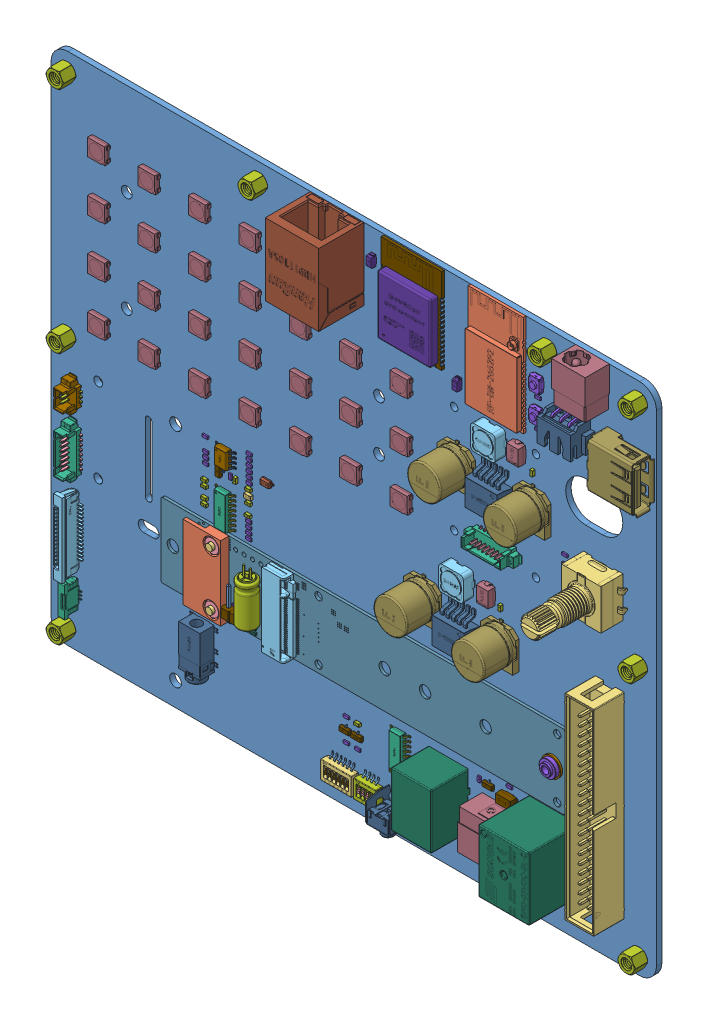
SolidWorks assembly HOUZZkitF1_Tester, configuration 默认. Lengths in mm. (continued)
Components (placement in the parent): (continued)
- HOUZZkitF1_Tester.step-1: HOUZZkitF1_Tester.step [默认] at origin size (180.06 153.05 26.45) (continued)
  - H4.step-1: H4.step [默认] at origin size (25.31 29.5 2.85) (continued)
    - tfcard_test_wire_female.step-1: tfcard_test_wire_female.step [默认] at (-76 20 -1.6) x (0 -1 0) z (0 0 -1) size (29.5 25.31 2.85) (continued)
      - MICRO SD CARD SOCKET.step-1: MICRO SD CARD SOCKET.step [默认] at (119.8236 -42.8675 -195.6897) size (16 17.9 2.44) (continued)
        - MICRO SD CARD SOCKET.step.step-1: MICRO SD CARD SOCKET.step.step [默认] at origin size (16 17.9 2.44) (continued)
          - MOV_SD-13.step.step-1: MOV_SD-13.step.step [默认] at origin size (1.3 1.09 0.1)
          - MOV_SD-14.step.step-1: MOV_SD-14.step.step [默认] at origin size (0.97 1.25 0.1)
          - MOV_SD-15.step.step-1: MOV_SD-15.step.step [默认] at origin size (0.18 0.18 0.1)
      - tfcard_test_wire_female-41.step-1: tfcard_test_wire_female-41.step [默认] at origin size (29.5 22.5 1)
  - LED1.step-1: LED1.step [默认] at origin size (5.4 5 1.7)
    - User Library-WS2812B.step-1: User Library-WS2812B.step [默认] at (-74.9999 93 0.18) x (1 0 0) z (0 -1 0) size (5.4 1.7 5)
  - H3.step-1: H3.step [默认] at origin size (120.05 22.08 8.14)
    - R44SF_bottom.step-1: R44SF_bottom.step [默认] at (-209.2275 115.0408 0.8) x (0 -1 0) z (0 0 1) size (22.08 120.05 8.14)
      - R44SF ..22.step.step-1: R44SF ..22.step.step [默认] at origin size (22.08 120.05 8.14)
        - Board.step.step-1: Board.step.step [默认] at origin size (22.05 120.05 0.8)
          - Open CASCADE STEP translator 6.8 12.1.1.step.step-1: Open CASCADE STEP translator 6.8 12.1.1.step.step [默认] at (0 0 -0.8) size (22.05 120.05 0.8)
        - R3.step.step-1: R3.step.step [默认] at origin size (1.6 0.8 0.45)
          - ________R0603.step.step-1: ________R0603.step.step [默认] at (119.5501 177.9636 0) x (1 0 0) z (0 0 1) size (1.6 0.8 0.45)
            - ________R0603-0.step.step-1: ________R0603-0.step.step [默认] at origin size (1.6 0.8 0.45)
        - D1.step.step-1: D1.step.step [默认] at origin size (0.8 1.6 1.1)
          - LED_AP1608.step.step-1: LED_AP1608.step.step [默认] at (120.3536 180.4092 0) x (0 1 0) z (1 0 0) size (1.6 1.1 0.8)
        - R2.step.step-1: R2.step.step [默认] at origin size (0.8 1.6 0.45)
          - ________R0603.step.step-1: ________R0603.step.step [默认] at (121.7526 180.421 0) x (0 -1 0) z (0 0 1) size (1.6 0.8 0.45)
            - ________R0603-0.step.step-1: ________R0603-0.step.step [默认] at origin size (1.6 0.8 0.45)
        - R1.step.step-1: R1.step.step [默认] at origin size (0.8 1.6 0.45)
          - ________R0603.step.step-1: ________R0603.step.step [默认] at (123.1496 180.421 0) x (0 -1 0) z (0 0 1) size (1.6 0.8 0.45)
            - ________R0603-0.step.step-1: ________R0603-0.step.step [默认] at origin size (1.6 0.8 0.45)
        - Q1.step.step-1: Q1.step.step [默认] at origin size (3 2.55 1)
          - SOT-23.step.step-1: SOT-23.step.step [默认] at (113.165 176.0289 0) x (-1 0 0) z (0 0 1) size (3 2.55 1)
        - Free-Models.step.step-1: Free-Models.step.step [默认] at origin size (22.05 110.48 8.14)
          - bg075-02x-1-0600-0300-0150-x-x_revd.step.step-1: bg075-02x-1-0600-0300-0150-x-x_revd.step.step [默认] at (120.1725 176.0952 0.5) x (0 -1 0) z (0 0 -1) size (5.08 10.36 5.5)
            - BG075-Insulator.step.step-1: BG075-Insulator.step.step [默认] at (0.3712 -0.9743 -0.1079) size (2.54 2.54 2.5)
            - BG075-Insulator.step.step-2: BG075-Insulator.step.step [默认] at (-2.1688 -0.9743 -0.1079) size (2.54 2.54 2.5)
            - BG075-1-0600-0300-0150-pin.step.step-1: BG075-1-0600-0300-0150-pin.step.step [默认] at (1.0892 -2.7943 -1.0379) size (0.64 10.36 4.57)
            - BG075-1-0600-0300-0150-pin.step.step-2: BG075-1-0600-0300-0150-pin.step.step [默认] at (-1.4508 -2.7943 -1.0379) size (0.64 10.36 4.57)
          - RP44S-PAD.step.step-1: RP44S-PAD.step.step [默认] at (102.0666 172.9244 2.5) x (-1 0 0) z (0 -1 0) size (22 2.5 11.2)
          - G0033_RGB9411503.step.step-1: G0033_RGB9411503.step.step [默认] at (121.2666 170.1244 -1.8) x (-1 0 0) z (0 1 0) size (3.3 5 3.3)
          - Hexagon_nut_ISO_4032_(DIN_934)_-_M2_RGB9411503.step.step-1: Hexagon_nut_ISO_4032_(DIN_934)_-_M2_RGB9411503.step.step [默认] at (121.2666 170.1244 1.5) x (-1 0 0) z (0 1 0) size (4.62 1.6 4.62)
          - Hexagon_nut_ISO_4032_(DIN_934)_-_M2_RGB9411503.step.step-2: Hexagon_nut_ISO_4032_(DIN_934)_-_M2_RGB9411503.step.step [默认] at (104.8666 170.1274 1.5) x (-1 0 0) z (0 1 0) size (4.62 1.6 4.62)
          - G0033_RGB9411503.step.step-2: G0033_RGB9411503.step.step [默认] at (104.8666 170.1274 -1.8) x (-1 0 0) z (0 1 0) size (3.3 5 3.3)
          - c-1-2199119-3-a1-3d_RGB4404530.step.step-1: c-1-2199119-3-a1-3d_RGB4404530.step.step [默认] at (113.0625 193.4584 1.7) x (-1 0 0) z (0 1 0) size (21.9 3.7 8.7)
          - Tape_22x5_RGB0.step.step-1: Tape_22x5_RGB0.step.step [默认] at (102.119 161.6272 -1) x (1 0 0) z (0 0 1) size (22 5 0.1)
          - CAP_RAD_D5x11_POL_BK.step.step-1: CAP_RAD_D5x11_POL_BK.step.step [默认] at (106.7892 181.2957 3) x (0 -1 0) z (1 0 0) size (5.5 5.5 15.01)
          - M2_nuc_RGB3326705.step.step-1: M2_nuc_RGB3326705.step.step [默认] at (113.0667 269.231 -1.1) x (1 0 0) z (0 -1 0) size (5 3.5 5)
          - G0042.step.step-1: G0042.step.step [默认] at (113.0667 269.231 0) x (1 0 0) z (0 -1 0) size (5.76 0.6 5.76)
          - G0042.step.step-2: G0042.step.step [默认] at (113.0667 269.231 -1.4) x (1 0 0) z (0 -1 0) size (5.76 0.6 5.76)
          - G0030_RGB12967653.step.step-1: G0030_RGB12967653.step.step [默认] at (113.0666 269.231 -1.9) x (1 0 0) z (0 -1 0) size (4.1 2.44 4.1)
  - USB2.step-1: USB2.step [默认] at origin size (14.31 14.74 11.11)
    - USB A__ __-1.step-1: USB A__ __-1.step [默认] at (76 90 0) x (0 1 0) z (0 0 1) size (14.74 14.3 11.11)
      - LOGO__-42.step-1: LOGO__-42.step [默认] at (-3.4255 -1.6966 0.196) x (-1 0 0) z (0 0 -1) size (1.2 1.38 0.01)
      - USB A__ __-1-43.step-1: USB A__ __-1-43.step [默认] at origin size (14.74 14.3 11.11)
  - J10.step-1: J10.step [默认] at origin size (10 12.1 10.2)
    - DC-044A-25A.step-1: DC-044A-25A.step [默认] at (43 -27.8499 0) x (1 0 0) z (0 -1 0) size (10 10.2 12.1)
  - USB1.step-1: USB1.step [默认] at origin size (13.84 16.3 14.4)
    - USB B__ __-1.step-1: USB B__ __-1.step [默认] at (28.5 -15 0) x (1 0 0) z (0 0 1) size (13.84 16.3 14.4)
      - LOGO__-44.step-1: LOGO__-44.step [默认] at (-1.3279 -1.8386 0.646) x (-1 0 0) z (0 0 -1) size (1.2 1.38 0.01)
      - USB B__ __-1-45.step-1: USB B__ __-1-45.step [默认] at origin size (13.84 16.3 14.4)
  - LED25.step-1: LED25.step [默认] at origin size (5.4 5 1.7)
    - User Library-WS2812B.step-1: User Library-WS2812B.step [默认] at (15.0001 48 0.18) x (1 0 0) z (0 -1 0) size (5.4 1.7 5)
  - LED24.step-1: LED24.step [默认] at origin size (5.4 5 1.7)
    - User Library-WS2812B.step-1: User Library-WS2812B.step [默认] at (0.0001 48 0.18) x (1 0 0) z (0 -1 0) size (5.4 1.7 5)
  - LED23.step-1: LED23.step [默认] at origin size (5.4 5 1.7)
    - User Library-WS2812B.step-1: User Library-WS2812B.step [默认] at (-14.9999 48 0.18) x (1 0 0) z (0 -1 0) size (5.4 1.7 5)
  - LED22.step-1: LED22.step [默认] at origin size (5.4 5 1.7)
    - User Library-WS2812B.step-1: User Library-WS2812B.step [默认] at (-29.9999 48 0.18) x (1 0 0) z (0 -1 0) size (5.4 1.7 5)
  - LED21.step-1: LED21.step [默认] at origin size (5.4 5 1.7)
    - User Library-WS2812B.step-1: User Library-WS2812B.step [默认] at (-44.9999 48 0.18) x (1 0 0) z (0 -1 0) size (5.4 1.7 5)
  - LED20.step-1: LED20.step [默认] at origin size (5.4 5 1.7)
    - User Library-WS2812B.step-1: User Library-WS2812B.step [默认] at (-59.9999 48 0.18) x (1 0 0) z (0 -1 0) size (5.4 1.7 5)
  - LED19.step-1: LED19.step [默认] at origin size (5.4 5 1.7)
    - User Library-WS2812B.step-1: User Library-WS2812B.step [默认] at (-74.9999 48 0.18) x (1 0 0) z (0 -1 0) size (5.4 1.7 5)
  - LED18.step-1: LED18.step [默认] at origin size (5.4 5 1.7)
    - User Library-WS2812B.step-1: User Library-WS2812B.step [默认] at (15.0001 63 0.18) x (1 0 0) z (0 -1 0) size (5.4 1.7 5)
  - LED17.step-1: LED17.step [默认] at origin size (5.4 5 1.7)
    - User Library-WS2812B.step-1: User Library-WS2812B.step [默认] at (0.0001 63 0.18) x (1 0 0) z (0 -1 0) size (5.4 1.7 5)
  - LED16.step-1: LED16.step [默认] at origin size (5.4 5 1.7)
    - User Library-WS2812B.step-1: User Library-WS2812B.step [默认] at (-14.9999 63 0.18) x (1 0 0) z (0 -1 0) size (5.4 1.7 5)
  - LED15.step-1: LED15.step [默认] at origin size (5.4 5 1.7)
    - User Library-WS2812B.step-1: User Library-WS2812B.step [默认] at (-29.9999 63 0.18) x (1 0 0) z (0 -1 0) size (5.4 1.7 5)
  - LED14.step-1: LED14.step [默认] at origin size (5.4 5 1.7)
    - User Library-WS2812B.step-1: User Library-WS2812B.step [默认] at (-44.9999 63 0.18) x (1 0 0) z (0 -1 0) size (5.4 1.7 5)
  - LED13.step-1: LED13.step [默认] at origin size (5.4 5 1.7)
    - User Library-WS2812B.step-1: User Library-WS2812B.step [默认] at (-59.9999 63 0.18) x (1 0 0) z (0 -1 0) size (5.4 1.7 5)
  - LED12.step-1: LED12.step [默认] at origin size (5.4 5 1.7)
    - User Library-WS2812B.step-1: User Library-WS2812B.step [默认] at (-74.9999 63 0.18) x (1 0 0) z (0 -1 0) size (5.4 1.7 5)
  - LED11.step-1: LED11.step [默认] at origin size (5.4 5 1.7)
    - User Library-WS2812B.step-1: User Library-WS2812B.step [默认] at (15.0001 78 0.18) x (1 0 0) z (0 -1 0) size (5.4 1.7 5)
  - LED10.step-1: LED10.step [默认] at origin size (5.4 5 1.7)
    - User Library-WS2812B.step-1: User Library-WS2812B.step [默认] at (0.0001 78 0.18) x (1 0 0) z (0 -1 0) size (5.4 1.7 5)
  - LED9.step-1: LED9.step [默认] at origin size (5.4 5 1.7)
    - User Library-WS2812B.step-1: User Library-WS2812B.step [默认] at (-14.9999 78 0.18) x (1 0 0) z (0 -1 0) size (5.4 1.7 5)
  - LED8.step-1: LED8.step [默认] at origin size (5.4 5 1.7)
    - User Library-WS2812B.step-1: User Library-WS2812B.step [默认] at (-29.9999 78 0.18) x (1 0 0) z (0 -1 0) size (5.4 1.7 5)
  - LED7.step-1: LED7.step [默认] at origin size (5.4 5 1.7)
    - User Library-WS2812B.step-1: User Library-WS2812B.step [默认] at (-44.9999 78 0.18) x (1 0 0) z (0 -1 0) size (5.4 1.7 5)
  - LED6.step-1: LED6.step [默认] at origin size (5.4 5 1.7)
    - User Library-WS2812B.step-1: User Library-WS2812B.step [默认] at (-59.9999 78 0.18) x (1 0 0) z (0 -1 0) size (5.4 1.7 5)
  - LED5.step-1: LED5.step [默认] at origin size (5.4 5 1.7)
    - User Library-WS2812B.step-1: User Library-WS2812B.step [默认] at (-74.9999 78 0.18) x (1 0 0) z (0 -1 0) size (5.4 1.7 5)
  - LED4.step-1: LED4.step [默认] at origin size (5.4 5 1.7)
    - User Library-WS2812B.step-1: User Library-WS2812B.step [默认] at (-29.9999 93 0.18) x (1 0 0) z (0 -1 0) size (5.4 1.7 5)
  - LED3.step-1: LED3.step [默认] at origin size (5.4 5 1.7)
    - User Library-WS2812B.step-1: User Library-WS2812B.step [默认] at (-44.9999 93 0.18) x (1 0 0) z (0 -1 0) size (5.4 1.7 5)
  - LED2.step-1: LED2.step [默认] at origin size (5.4 5 1.7)
    - User Library-WS2812B.step-1: User Library-WS2812B.step [默认] at (-59.9999 93 0.18) x (1 0 0) z (0 -1 0) size (5.4 1.7 5)
  - U2.step-1: U2.step [默认] at origin size (18.02 25.51 3.16)
    - ESP32-S3-WROOM-1.step-1: ESP32-S3-WROOM-1.step [默认] at (18 100 0.1) x (1 0 0) z (0 -1 0) size (18.02 3.16 25.51)
      - ESP-S3-WROOM_via v3.step-1: ESP-S3-WROOM_via v3.step [默认] at (-9.01 -0.05 11.25) size (0.85 0.9 0.9)
      - ESP32-S3-WROOM_shell v11.step-1: ESP32-S3-WROOM_shell v11.step [默认] at (0 0.8 2.9) size (15.8 2.31 17.6)
      - ESP32-S3-WROOM_body v12.step-1: ESP32-S3-WROOM_body v12.step [默认] at origin size (18 0.84 25.5)
      - ESP-S3-WROOM_via v3.step-2: ESP-S3-WROOM_via v3.step [默认] at (-9.01 -0.05 9.98) size (0.85 0.9 0.9)
      - ESP-S3-WROOM_via v3.step-3: ESP-S3-WROOM_via v3.step [默认] at (-9.01 -0.05 8.71) size (0.85 0.9 0.9)
      - ESP-S3-WROOM_via v3.step-4: ESP-S3-WROOM_via v3.step [默认] at (-9.01 -0.05 7.44) size (0.85 0.9 0.9)
      - ESP-S3-WROOM_via v3.step-5: ESP-S3-WROOM_via v3.step [默认] at (-9.01 -0.05 6.17) size (0.85 0.9 0.9)
      - ESP-S3-WROOM_via v3.step-6: ESP-S3-WROOM_via v3.step [默认] at (-9.01 -0.05 4.9) size (0.85 0.9 0.9)
      - ESP-S3-WROOM_via v3.step-7: ESP-S3-WROOM_via v3.step [默认] at (-9.01 -0.05 3.63) size (0.85 0.9 0.9)
      - ESP-S3-WROOM_via v3.step-8: ESP-S3-WROOM_via v3.step [默认] at (-9.01 -0.05 2.36) size (0.85 0.9 0.9)
      - ESP-S3-WROOM_via v3.step-9: ESP-S3-WROOM_via v3.step [默认] at (-9.01 -0.05 1.09) size (0.85 0.9 0.9)
      - ESP-S3-WROOM_via v3.step-10: ESP-S3-WROOM_via v3.step [默认] at (-9.01 -0.05 -0.18) size (0.85 0.9 0.9)
      - ESP-S3-WROOM_via v3.step-11: ESP-S3-WROOM_via v3.step [默认] at (-9.01 -0.05 -1.45) size (0.85 0.9 0.9)
      - ESP-S3-WROOM_via v3.step-12: ESP-S3-WROOM_via v3.step [默认] at (-9.01 -0.05 -2.72) size (0.85 0.9 0.9)
      - ESP-S3-WROOM_via v3.step-13: ESP-S3-WROOM_via v3.step [默认] at (-9.01 -0.05 -3.99) size (0.85 0.9 0.9)
      - ESP-S3-WROOM_via v3.step-14: ESP-S3-WROOM_via v3.step [默认] at (-9.01 -0.05 -5.26) size (0.85 0.9 0.9)
      - ESP-S3-WROOM_via v3(______).step-1: ESP-S3-WROOM_via v3(______).step [默认] at (9.01 -0.05 11.25) x (-1 0 0) z (0 0 -1) size (0.85 0.9 0.9)
      - ESP-S3-WROOM_via v3(______).step-2: ESP-S3-WROOM_via v3(______).step [默认] at (9.01 -0.05 9.98) x (-1 0 0) z (0 0 -1) size (0.85 0.9 0.9)
      - ESP-S3-WROOM_via v3(______).step-3: ESP-S3-WROOM_via v3(______).step [默认] at (9.01 -0.05 8.71) x (-1 0 0) z (0 0 -1) size (0.85 0.9 0.9)
      - ESP-S3-WROOM_via v3(______).step-4: ESP-S3-WROOM_via v3(______).step [默认] at (9.01 -0.05 7.44) x (-1 0 0) z (0 0 -1) size (0.85 0.9 0.9)
      - ESP-S3-WROOM_via v3(______).step-5: ESP-S3-WROOM_via v3(______).step [默认] at (9.01 -0.05 6.17) x (-1 0 0) z (0 0 -1) size (0.85 0.9 0.9)
      - ESP-S3-WROOM_via v3(______).step-6: ESP-S3-WROOM_via v3(______).step [默认] at (9.01 -0.05 4.9) x (-1 0 0) z (0 0 -1) size (0.85 0.9 0.9)
      - ESP-S3-WROOM_via v3(______).step-7: ESP-S3-WROOM_via v3(______).step [默认] at (9.01 -0.05 3.63) x (-1 0 0) z (0 0 -1) size (0.85 0.9 0.9)
      - ESP-S3-WROOM_via v3(______).step-8: ESP-S3-WROOM_via v3(______).step [默认] at (9.01 -0.05 2.36) x (-1 0 0) z (0 0 -1) size (0.85 0.9 0.9)
      - ESP-S3-WROOM_via v3(______).step-9: ESP-S3-WROOM_via v3(______).step [默认] at (9.01 -0.05 1.09) x (-1 0 0) z (0 0 -1) size (0.85 0.9 0.9)
      - ESP-S3-WROOM_via v3(______).step-10: ESP-S3-WROOM_via v3(______).step [默认] at (9.01 -0.05 -0.18) x (-1 0 0) z (0 0 -1) size (0.85 0.9 0.9)
      - ESP-S3-WROOM_via v3(______).step-11: ESP-S3-WROOM_via v3(______).step [默认] at (9.01 -0.05 -1.45) x (-1 0 0) z (0 0 -1) size (0.85 0.9 0.9)
      - ESP-S3-WROOM_via v3(______).step-12: ESP-S3-WROOM_via v3(______).step [默认] at (9.01 -0.05 -2.72) x (-1 0 0) z (0 0 -1) size (0.85 0.9 0.9)
      - ESP-S3-WROOM_via v3(______).step-13: ESP-S3-WROOM_via v3(______).step [默认] at (9.01 -0.05 -3.99) x (-1 0 0) z (0 0 -1) size (0.85 0.9 0.9)
      - ESP-S3-WROOM_via v3(______).step-14: ESP-S3-WROOM_via v3(______).step [默认] at (9.01 -0.05 -5.26) x (-1 0 0) z (0 0 -1) size (0.85 0.9 0.9)
      - ESP-S3-WROOM_via v3.step-15: ESP-S3-WROOM_via v3.step [默认] at (-6.985 -0.05 12.76) x (0 0 -1) z (1 0 0) size (0.85 0.9 0.9)
      - ESP-S3-WROOM_via v3.step-16: ESP-S3-WROOM_via v3.step [默认] at (-5.715 -0.05 12.76) x (0 0 -1) z (1 0 0) size (0.85 0.9 0.9)
      - ESP-S3-WROOM_via v3.step-17: ESP-S3-WROOM_via v3.step [默认] at (-4.445 -0.05 12.76) x (0 0 -1) z (1 0 0) size (0.85 0.9 0.9)
      - ESP-S3-WROOM_via v3.step-18: ESP-S3-WROOM_via v3.step [默认] at (-3.175 -0.05 12.76) x (0 0 -1) z (1 0 0) size (0.85 0.9 0.9)
      - ESP-S3-WROOM_via v3.step-19: ESP-S3-WROOM_via v3.step [默认] at (-1.905 -0.05 12.76) x (0 0 -1) z (1 0 0) size (0.85 0.9 0.9)
      - ESP-S3-WROOM_via v3.step-20: ESP-S3-WROOM_via v3.step [默认] at (-0.635 -0.05 12.76) x (0 0 -1) z (1 0 0) size (0.85 0.9 0.9)
      - ESP-S3-WROOM_via v3.step-21: ESP-S3-WROOM_via v3.step [默认] at (0.635 -0.05 12.76) x (0 0 -1) z (1 0 0) size (0.85 0.9 0.9)
      - ESP-S3-WROOM_via v3.step-22: ESP-S3-WROOM_via v3.step [默认] at (1.905 -0.05 12.76) x (0 0 -1) z (1 0 0) size (0.85 0.9 0.9)
      - ESP-S3-WROOM_via v3.step-23: ESP-S3-WROOM_via v3.step [默认] at (3.175 -0.05 12.76) x (0 0 -1) z (1 0 0) size (0.85 0.9 0.9)
      - ESP-S3-WROOM_via v3.step-24: ESP-S3-WROOM_via v3.step [默认] at (4.445 -0.05 12.76) x (0 0 -1) z (1 0 0) size (0.85 0.9 0.9)
      - ESP-S3-WROOM_via v3.step-25: ESP-S3-WROOM_via v3.step [默认] at (5.715 -0.05 12.76) x (0 0 -1) z (1 0 0) size (0.85 0.9 0.9)
      - ESP-S3-WROOM_via v3.step-26: ESP-S3-WROOM_via v3.step [默认] at (6.985 -0.05 12.76) x (0 0 -1) z (1 0 0) size (0.85 0.9 0.9)
  - U1.step-1: U1.step [默认] at origin size (16.4 30 2.21)
    - RF-BM-2652P2.step-1: RF-BM-2652P2.step [默认] at (42.9964 98 0) x (1 0 0) z (0 -1 0) size (16.4 2.21 30)
  - SW1.step-1: SW1.step [默认] at origin size (14.8 12.49 25.5)
    - CE11.step-1: CE11.step [默认] at (74.2 55 0) x (1 0 0) z (0 0 1) size (14.8 12.49 25.5)
      - CE11-46.step-1: CE11-46.step [默认] x (1 0 0) z (0 -1 0) size (14.8 25.5 12.49)
      - LOGO__-47.step-1: LOGO__-47.step [默认] at (0.0178 0.3286 -0.012) x (-1 0 0) z (0 0 -1) size (3.6 4.15 0.02)
  - JP5.step-1: JP5.step [默认] at origin size (4.5 22.1 5.4)
    - FPC1.0-15P-LI.step-1: FPC1.0-15P-LI.step [默认] at (-74.5498 -5.5498 -1.5) x (0 -1 0) z (0 0 1) size (22.1 4.5 5.4)
      - 3D_PCB1_2022-09-05.step.step-1: 3D_PCB1_2022-09-05.step.step [默认] at origin size (22.1 4.5 5.4)
        - FPC1.step.step-1: FPC1.step.step [默认] at (2.9502 -7.9502 1.6001) size (22.1 4.5 5.4)
          - FPC-SMD_15P-P1.00_HDGC_1.0K-GT-15PB.step.step-1: FPC-SMD_15P-P1.00_HDGC_1.0K-GT-15PB.step.step [默认] at origin size (22.1 4.5 5.4)
            - =_[0_1_1_5].step.step-1: =_[0_1_1_5].step.step [默认] at origin size (22.1 4.5 5.4)
  - JP3.step-1: JP3.step [默认] at origin size (3.5 9.15 4.5)
    - 0.5K-A-7PB.step-1: 0.5K-A-7PB.step [默认] at (-77.2346 -24.45 -1.55) x (0 -1 0) z (0 0 1) size (9.15 3.5 4.5)
      - 3D_PCB1_2022-11-23.step.step-1: 3D_PCB1_2022-11-23.step.step [默认] at origin size (9.15 3.5 4.5)
        - FPC2.step.step-1: FPC2.step.step [默认] at (0.53 -5.2454 1.6) size (9.15 3.5 4.5)
          - FPC-SMD_7P-P0.50_HDGC_0.5K-A-7PB.step.step-1: FPC-SMD_7P-P0.50_HDGC_0.5K-A-7PB.step.step [默认] at origin size (9.15 3.5 4.5)
            - COMPOUND.step-48.step-1: COMPOUND.step-48.step [默认] at origin size (9.15 3.5 4.5)
  - JP2.step-1: JP2.step [默认] at origin size (4.1 15.15 4.7)
    - MOLEX1.25-LS-8P.step-1: MOLEX1.25-LS-8P.step [默认] at (-83 12 0) x (0 1 0) z (0 0 1) size (15.15 4.1 4.7)
      - MOLEX1.25-LS-______.step-1: MOLEX1.25-LS-______.step [默认] at (4.375 0.45 0.75) x (0 -1 0) z (0 0 1) size (3.7 0.32 3.85)
      - MOLEX1.25-LS-______.step-2: MOLEX1.25-LS-______.step [默认] at (3.125 0.45 0.75) x (0 -1 0) z (0 0 1) size (3.7 0.32 3.85)
      - MOLEX1.25-LS-______.step-3: MOLEX1.25-LS-______.step [默认] at (1.875 0.45 0.75) x (0 -1 0) z (0 0 1) size (3.7 0.32 3.85)
      - MOLEX1.25-LS-______.step-4: MOLEX1.25-LS-______.step [默认] at (0.625 0.45 0.75) x (0 -1 0) z (0 0 1) size (3.7 0.32 3.85)
      - MOLEX1.25-LS-______.step-5: MOLEX1.25-LS-______.step [默认] at (-0.625 0.45 0.75) x (0 -1 0) z (0 0 1) size (3.7 0.32 3.85)
      - MOLEX1.25-LS-______.step-6: MOLEX1.25-LS-______.step [默认] at (-1.875 0.45 0.75) x (0 -1 0) z (0 0 1) size (3.7 0.32 3.85)
      - MOLEX1.25-LS-______.step-7: MOLEX1.25-LS-______.step [默认] at (-3.125 0.45 0.75) x (0 -1 0) z (0 0 1) size (3.7 0.32 3.85)
      - MOLEX1.25-LS-______.step-8: MOLEX1.25-LS-______.step [默认] at (-4.375 0.45 0.75) x (0 -1 0) z (0 0 1) size (3.7 0.32 3.85)
      - LOGO__0.15-37.step-1: LOGO__0.15-37.step [默认] at (5.035 0.4556 0.247) size (0.45 0.52 0)
      - MOLEX1.25-LS-8P-38.step-1: MOLEX1.25-LS-8P-38.step [默认] at origin size (15.15 3.6 4.7)
  - JP1.step-1: JP1.step [默认] at origin size (4.1 8.9 4.7)
    - MOLEX1.25-LS-3P.step-1: MOLEX1.25-LS-3P.step [默认] at (-83 26.247 0) x (0 1 0) z (0 0 1) size (8.9 4.1 4.7)
      - MOLEX1.25-LS-______-49.step-1: MOLEX1.25-LS-______-49.step [默认] at (1.25 0.45 0.75) x (0 -1 0) z (0 0 1) size (3.7 0.32 3.85)
      - MOLEX1.25-LS-______-49.step-2: MOLEX1.25-LS-______-49.step [默认] at (0 0.45 0.75) x (0 -1 0) z (0 0 1) size (3.7 0.32 3.85)
      - MOLEX1.25-LS-______-49.step-3: MOLEX1.25-LS-______-49.step [默认] at (-1.25 0.45 0.75) x (0 -1 0) z (0 0 1) size (3.7 0.32 3.85)
      - LOGO__0.15-50.step-1: LOGO__0.15-50.step [默认] at (1.91 0.4556 0.247) size (0.45 0.52 0)
      - MOLEX1.25-LS-3P-51.step-1: MOLEX1.25-LS-3P-51.step [默认] at origin size (8.9 3.6 4.7)
  - J3.step-1: J3.step [默认] at origin size (10 12.1 10.2)
    - DC-044A-25A.step-1: DC-044A-25A.step [默认] at (71 112.8499 0) x (-1 0 0) z (0 1 0) size (10 10.2 12.1)
  - CON1.step-1: CON1.step [默认] at origin size (8.3 14.1 5.3)
    - PJ342A.step-1: PJ342A.step [默认] at (-44.5 -22.6 -0.05) x (-1 0 0) z (0 0 1) size (8.3 14.1 5.3)
      - PJ342A-52.step-1: PJ342A-52.step [默认] at origin size (8.3 14.1 5.3)
      - LOGO__0.5-53.step-1: LOGO__0.5-53.step [默认] at (0 -2.992 0.045) x (-1 0 0) z (0 0 -1) size (1.5 1.73 0.01)
